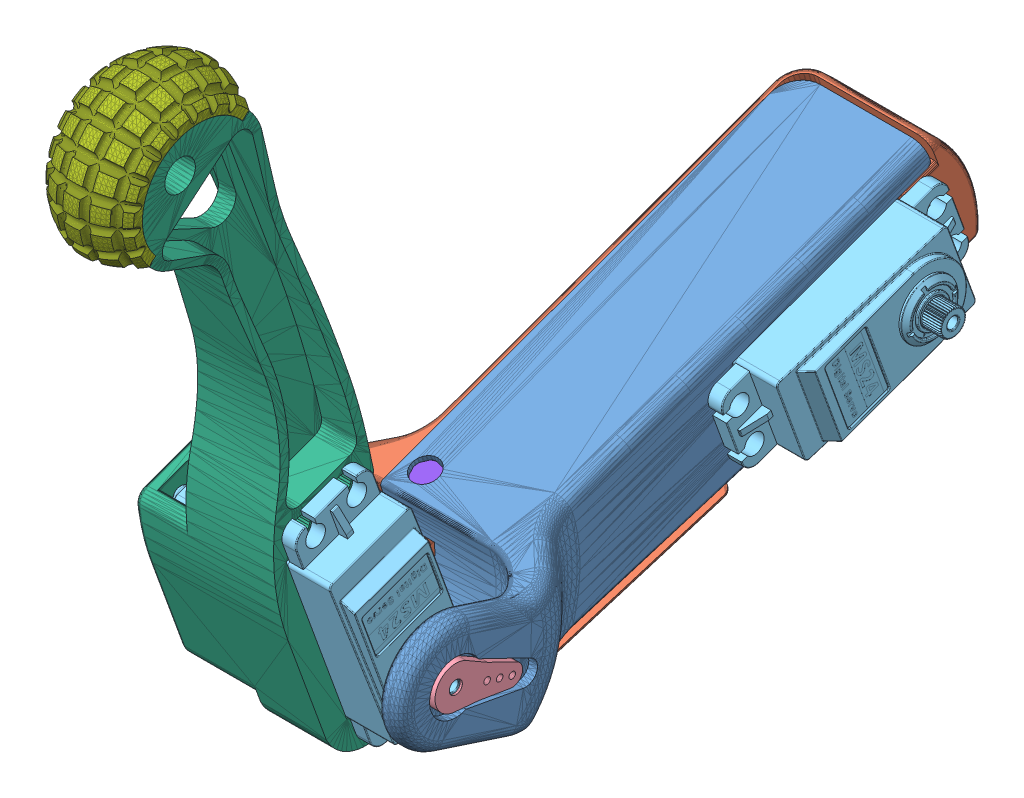
SolidWorks assembly Right Leg Assembly, configuration Default. Lengths in mm.
Overall size (64.22 167.45 199.81).
25 component instances, 9 part files, 59 mates.
Components (placement in the parent):
- Right_arm_joint_mg-1: Right_arm_joint_mg [Default] at (24.2858 18.5405 -25.0321) size (37.5 46 56.5) (hidden)
- Servohorn-1: Servohorn [4 Prong] at (-38.4142 28.7905 -4.7821) x (0 0.715501 0.698611) z (-1 0 0) size (31.8 31.8 2.24) (hidden)
- Servo Motor-1: Servo Motor [Default] at (-15.7142 38.5405 -14.5321) size (20.1 45.99 55.6) (hidden)
- Servohorn-2: Servohorn [Default] at (-15.7142 58.9405 -14.5321) x (-0.99999 0 0.00451) z (0 -1 0) size (28.18 31.8 2.24) (hidden)
- Right_arm_mg-1: Right_arm_mg [Default] at (-8.8142 41.6076 -10.7588) x (0 -0.939693 -0.34202) z (0 -0.34202 0.939693) size (38.24 39.8 137.4)
- SM_Right_arm_cover-1: SM_Right_arm_cover [Default] at (-48.6142 49.0427 -16.5661) x (0 -0.939693 -0.34202) z (0 -0.34202 0.939693) size (41.16 45 143.55)
- F625ZZ Ball Bearing-1: F625ZZ Ball Bearing [Default] at (-98.6142 -2.6723 100.0196) x (0 0.0383 -0.999266) z (1 0 0) size (18 18 5)
- Servohorn-3: Servohorn [1 Prong] at (-48.8142 5.2058 100.4211) x (0 -0.953491 0.301422) z (-1 0 0) size (9.55 20.65 2.24)
- Servo Motor-2: Servo Motor [Default] at (-67.7142 5.2058 100.4211) x (0 -0.34202 0.939693) z (0 0.939693 0.34202) size (20.1 45.99 55.6)
- Servo Motor-3: Servo Motor [Default] at (-58.8142 28.7905 -4.7821) x (0 -0.939693 -0.34202) z (0 -0.34202 0.939693) size (20.1 45.99 55.6)
- Right_wrist_mg-1: Right_wrist_mg [Default] at (-67.7142 -0.7709 87.604) x (0 0.939693 0.34202) z (0 -0.34202 0.939693) size (149.99 36.9 30)
- foot-1: foot [Default] at (-67.7142 114.2242 140.0873) x (0 -0.656061 0.754708) z (0 -0.754708 -0.656061) size (38.32 20 19.41)
- _Hex_Screws-1: _Hex_Screws [H M4x20] at (-20.7142 41.7405 19.4679) x (-0.837169 0 -0.546944) z (-0.546944 0 0.837169) size (7 22.8 8.08) (hidden)
- _Hex_Screws-2: _Hex_Screws [H M4x20] at (-10.7142 41.7405 -28.5321) x (-0.837169 0 -0.546944) z (-0.546944 0 0.837169) size (7 22.8 8.08) (hidden)
- _Hex_Screws-3: _Hex_Screws [H M4x20] at (-10.7142 41.7405 19.4679) x (-0.99108 0 -0.133267) z (-0.133267 0 0.99108) size (7 22.8 8.08) (hidden)
- _Hex_Screws-4: _Hex_Screws [H M4x20] at (-20.7142 41.7405 -28.5321) x (0.837169 0 0.546944) z (0.546944 0 -0.837169) size (7 22.8 8.08) (hidden)
- _Hex_Screws-5: _Hex_Screws [H M4x20] at (-55.6142 28.8803 -19.6479) x (0 0.085299 -0.996355) z (0 0.996355 0.085299) size (7 22.8 8.08) (hidden)
- _Hex_Screws-8: _Hex_Screws [H M4x20] at (-55.6142 12.4633 25.4573) x (0 -0.381849 0.924225) z (0 -0.924225 -0.381849) size (7 22.8 8.08) (hidden)
- _Hex_Screws-9: _Hex_Screws [H M4x20] at (-55.6142 21.8603 28.8775) x (0 -0.381849 0.924225) z (0 -0.924225 -0.381849) size (7 22.8 8.08) (hidden)
- _Hex_Screws-10: _Hex_Screws [H M4x20] at (-64.5142 -9.66 100.3313) x (0 -0.381849 0.924225) z (0 -0.924225 -0.381849) size (7 22.8 8.08) (hidden)
- _Hex_Screws-11: _Hex_Screws [H M4x20] at (-64.5142 38.8655 107.3514) x (0 -0.381849 0.924225) z (0 -0.924225 -0.381849) size (7 22.8 8.08) (hidden)
- _Hex_Screws-12: _Hex_Screws [H M4x20] at (-64.5142 -6.2398 90.9344) x (0 -0.381849 0.924225) z (0 -0.924225 -0.381849) size (7 22.8 8.08) (hidden)
- _Hex_Screws-14: _Hex_Screws [H M4x20] at (-64.5142 35.4453 116.7483) x (0 -0.381849 0.924225) z (0 -0.924225 -0.381849) size (7 22.8 8.08) (hidden)
- _Hex_Screws-15: _Hex_Screws [H M4x20] at (-55.6142 38.2772 -16.2277) x (0 0.381849 -0.924225) z (0 0.924225 0.381849) size (7 22.8 8.08) (hidden)
- _Hex_Screws-19: _Hex_Screws [H M3x16] at (-83.8911 13.8209 71.432) x (0.19625 0.335369 -0.921419) z (-0.980554 0.067122 -0.184415) size (5.5 18 6.35)
Mates (geometry in assembly coordinates):
- Coincident1: coincident anti-aligned: plane of Right_arm_joint_mg-1 through (-40.4142 18.5405 -25.0321) normal (1 0 0); plane of Servohorn-1 through (-40.4142 28.7905 -4.7821) normal (-1 0 0)
- Angle2: planar angle = 0.069813 rad anti-aligned: plane of Right_arm_joint_mg-1 through (24.2858 29.9404 -17.8834) normal (0 0.847204 0.531268); plane of Servohorn-1 through (-40.4142 21.752 -2.4794) normal (0 -0.808081 -0.589071)
- Coincident4: coincident: point of Right_arm_joint_mg-1; line of Servohorn-1 through (-38.4142 28.7905 -4.7821) axis (1 0 0)
- Coincident5: coincident anti-aligned: plane of Right_arm_joint_mg-1 through (-25.7142 18.5405 -25.0321) normal (1 0 0); plane of Servo Motor-1 through (-25.7142 49.5405 -23.5321) normal (-1 0 0)
- Coincident6: coincident anti-aligned: plane of Right_arm_joint_mg-1 through (24.2858 11.0405 -25.0321) normal (0 1 0); plane of Servo Motor-1 through (-15.7142 11.0405 -14.5321) normal (0 -1 0)
- Distance2: distance = 0 mm anti-aligned: plane of Servo Motor-1 through (-25.7142 18.5405 15.4679) normal (0 0 1); plane of Right_arm_joint_mg-1 through (24.2858 18.5405 15.4679) normal (0 0 -1)
- Concentric1: concentric anti-aligned: cylinder of Servo Motor-1 through (-15.7142 52.9405 -14.5321) axis (0 1 0) radius 1.25; line of Servohorn-2 through (-15.7142 58.9405 -14.5321) axis (0 -1 0)
- Coincident8: coincident anti-aligned: plane of Servo Motor-1 through (-15.7142 56.9405 -14.5321) normal (0 1 0); plane of Servohorn-2 through (-15.7142 56.9405 -14.5321) normal (0 -1 0)
- Coincident14: coincident anti-aligned: plane of Right_arm_mg-1 through (-88.6142 41.6076 -10.7588) normal (-1 0 0); plane of SM_Right_arm_cover-1 through (-88.6142 49.0427 -16.5661) normal (1 0 0)
- Distance4: distance = 1 mm aligned: plane of Right_arm_mg-1 through (-8.8142 41.6076 -10.7588) normal (0 -0.34202 0.939693); plane of SM_Right_arm_cover-1 through (-48.6142 46.6485 -9.9883) normal (0 -0.34202 0.939693)
- Coincident16: coincident aligned: plane of Right_arm_mg-1 through (-8.8142 20.9865 -18.2643) normal (0 -0.939693 -0.34202); plane of SM_Right_arm_cover-1 through (-48.6142 23.7227 -25.7819) normal (0 -0.939693 -0.34202)
- Tangent1: tangent anti-aligned: plane of SM_Right_arm_cover-1 through (-58.6142 8.2907 92.877) normal (0 -0.30578 0.952102); cylinder of F625ZZ Ball Bearing-1 through (-101.6142 5.3219 100.326) axis (-1 0 0) radius 8
- Coincident17: coincident anti-aligned: plane of SM_Right_arm_cover-1 through (-99.6142 49.0427 -16.5661) normal (1 0 0); plane of F625ZZ Ball Bearing-1 through (-99.6142 13.316 100.6324) normal (-1 0 0)
- Tangent4: tangent anti-aligned: plane of SM_Right_arm_cover-1 through (-58.6142 13.3121 99.5229) normal (0 -0.98251 0.186209); cylinder of F625ZZ Ball Bearing-1 through (-101.6142 5.3219 100.326) axis (-1 0 0) radius 8
- Coincident18: coincident anti-aligned: plane of Right_arm_mg-1 through (-50.8142 41.6076 -10.7588) normal (1 0 0); plane of Servohorn-3 through (-50.8142 5.2058 100.4211) normal (-1 0 0)
- Coincident19: coincident: point of Right_arm_mg-1; line of Servohorn-3 through (-48.8142 5.2058 100.4211) axis (-1 0 0)
- Parallel3: parallel anti-aligned: plane of Right_arm_mg-1 through (-8.8142 -26.9471 22.3339) normal (0 -0.900565 0.434721); plane of Servohorn-3 through (-50.8142 6.495 93.1286) normal (0 0.900565 -0.434721)
- Concentric2: concentric anti-aligned: line of Servohorn-1 through (-38.4142 28.7905 -4.7821) axis (-1 0 0); cylinder of Servo Motor-3 through (-44.4142 28.7905 -4.7821) axis (1 0 0) radius 1.25
- Coincident21: coincident anti-aligned: plane of Servohorn-1 through (-40.4142 28.7905 -4.7821) normal (-1 0 0); plane of Servo Motor-3 through (-40.4142 28.7905 -4.7821) normal (1 0 0)
- Coincident23: coincident anti-aligned: plane of Right_arm_mg-1 through (-8.8142 41.6076 -10.7588) normal (0 -0.939693 -0.34202); plane of Servo Motor-3 through (-47.8142 41.2656 -9.8191) normal (0 0.939693 0.34202)
- Coincident24: coincident anti-aligned: plane of Right_arm_mg-1 through (-8.8142 41.6076 -10.7588) normal (0 -0.34202 0.939693); plane of Servo Motor-3 through (-78.8142 41.6076 -10.7588) normal (0 0.34202 -0.939693)
- Coincident25: coincident anti-aligned: plane of Right_arm_mg-1 through (-58.8142 41.6076 -10.7588) normal (1 0 0); plane of Servo Motor-3 through (-58.8142 11.0987 17.5114) normal (-1 0 0)
- Coincident26: coincident anti-aligned: plane of Servo Motor-2 through (-67.7142 27.4993 118.1129) normal (-1 0 0); plane of Right_wrist_mg-1 through (-67.7142 -0.7709 87.604) normal (1 0 0)
- Coincident27: coincident anti-aligned: plane of Servo Motor-2 through (-87.7142 -0.7709 87.604) normal (0 -0.939693 -0.34202); plane of Right_wrist_mg-1 through (-67.7142 -0.7709 87.604) normal (0 0.939693 0.34202)
- Coincident29: coincident anti-aligned: plane of Servo Motor-2 through (-56.7142 29.0367 119.7367) normal (0 -0.34202 0.939693); plane of Right_wrist_mg-1 through (-67.7142 -7.6113 106.3979) normal (0 0.34202 -0.939693)
- Concentric3: concentric aligned: line of Servohorn-3 through (-48.8142 5.2058 100.4211) axis (1 0 0); cylinder of Servo Motor-2 through (-53.3142 5.2058 100.4211) axis (1 0 0) radius 1.25
- Distance6: distance = 1.5 mm anti-aligned: plane of Servohorn-3 through (-50.8142 5.2058 100.4211) normal (-1 0 0); plane of Servo Motor-2 through (-49.3142 5.2058 100.4211) normal (1 0 0)
- Coincident31: coincident anti-aligned: plane of Right_wrist_mg-1 through (-67.7142 50.7034 176.7608) normal (0 -0.499997 -0.866027); plane of foot-1 through (-67.7142 114.2242 140.0873) normal (0 0.499997 0.866027)
- Coincident32: coincident aligned: plane of Right_wrist_mg-1 through (-87.7142 -0.7709 87.604) normal (-1 0 0); plane of foot-1 through (-87.7142 114.2242 140.0873) normal (-1 0 0)
- Coincident34: coincident: point of Right_wrist_mg-1; line of foot-1 through (-87.7142 124.0354 148.6161) axis (0 0.629912 -0.776667)
- Concentric4: concentric aligned: cylinder of Servo Motor-1 through (-10.7142 32.1765 19.4679) axis (0 1 0) radius 2.25; cylinder of _Hex_Screws-3 through (-10.7142 21.7405 19.4679) axis (0 1 0) radius 2
- Coincident35: coincident anti-aligned: plane of Servo Motor-1 through (-15.7142 41.7405 -14.5321) normal (0 1 0); plane of _Hex_Screws-3 through (-10.7142 41.7405 19.4679) normal (0 -1 0)
- Concentric5: concentric aligned: cylinder of Servo Motor-1 through (-20.7142 32.1765 19.4679) axis (0 1 0) radius 2.25; cylinder of _Hex_Screws-1 through (-20.7142 21.7405 19.4679) axis (0 1 0) radius 2
- Coincident36: coincident aligned: plane of _Hex_Screws-1 through (-20.7142 44.5405 19.4679) normal (0 1 0); plane of _Hex_Screws-3 through (-10.7142 44.5405 19.4679) normal (0 1 0)
- Concentric6: concentric aligned: cylinder of Servo Motor-1 through (-20.7142 32.1765 -28.5321) axis (0 1 0) radius 2.25; cylinder of _Hex_Screws-4 through (-20.7142 21.7405 -28.5321) axis (0 1 0) radius 2
- Coincident37: coincident anti-aligned: plane of Servo Motor-1 through (-15.7142 41.7405 -14.5321) normal (0 1 0); plane of _Hex_Screws-4 through (-20.7142 41.7405 -28.5321) normal (0 -1 0)
- Concentric7: concentric aligned: cylinder of Servo Motor-1 through (-10.7142 32.1765 -28.5321) axis (0 1 0) radius 2.25; cylinder of _Hex_Screws-2 through (-10.7142 21.7405 -28.5321) axis (0 1 0) radius 2
- Coincident38: coincident anti-aligned: plane of Servo Motor-1 through (-15.7142 41.7405 -14.5321) normal (0 1 0); plane of _Hex_Screws-2 through (-10.7142 41.7405 -28.5321) normal (0 -1 0)
- Concentric8: concentric aligned: cylinder of Servo Motor-3 through (-65.1781 12.4633 25.4573) axis (1 0 0) radius 2.25; cylinder of _Hex_Screws-8 through (-75.6142 12.4633 25.4573) axis (1 0 0) radius 2
- Coincident39: coincident anti-aligned: plane of Servo Motor-3 through (-55.6142 28.7905 -4.7821) normal (1 0 0); plane of _Hex_Screws-8 through (-55.6142 12.4633 25.4573) normal (-1 0 0)
- Concentric9: concentric aligned: cylinder of Servo Motor-3 through (-65.1781 21.8603 28.8775) axis (1 0 0) radius 2.25; cylinder of _Hex_Screws-9 through (-75.6142 21.8603 28.8775) axis (1 0 0) radius 2
- Coincident40: coincident aligned: plane of _Hex_Screws-8 through (-52.8142 12.4633 25.4573) normal (1 0 0); plane of _Hex_Screws-9 through (-52.8142 21.8603 28.8775) normal (1 0 0)
- Concentric10: concentric aligned: cylinder of Servo Motor-3 through (-65.1781 28.8803 -19.6479) axis (1 0 0) radius 2.25; cylinder of _Hex_Screws-5 through (-75.6142 28.8803 -19.6479) axis (1 0 0) radius 2
- Coincident41: coincident anti-aligned: plane of Servo Motor-3 through (-55.6142 28.7905 -4.7821) normal (1 0 0); plane of _Hex_Screws-5 through (-55.6142 28.8803 -19.6479) normal (-1 0 0)
- Coincident42: coincident aligned: plane of _Hex_Screws-5 through (-52.8142 28.8803 -19.6479) normal (1 0 0); plane of _Hex_Screws-15 through (-52.8142 38.2772 -16.2277) normal (1 0 0)
- Concentric11: concentric aligned: cylinder of Servo Motor-3 through (-65.1781 38.2772 -16.2277) axis (1 0 0) radius 2.25; cylinder of _Hex_Screws-15 through (-75.6142 38.2772 -16.2277) axis (1 0 0) radius 2
- Concentric12: concentric aligned: cylinder of Servo Motor-2 through (-74.0781 38.8655 107.3514) axis (1 0 0) radius 2.25; cylinder of _Hex_Screws-11 through (-84.5142 38.8655 107.3514) axis (1 0 0) radius 2
- Concentric13: concentric aligned: cylinder of Servo Motor-2 through (-74.0781 35.4453 116.7483) axis (1 0 0) radius 2.25; cylinder of _Hex_Screws-14 through (-84.5142 35.4453 116.7483) axis (1 0 0) radius 2
- Concentric14: concentric aligned: cylinder of Servo Motor-2 through (-74.0781 -6.2398 90.9344) axis (1 0 0) radius 2.25; cylinder of _Hex_Screws-12 through (-84.5142 -6.2398 90.9344) axis (1 0 0) radius 2
- Concentric15: concentric aligned: cylinder of Servo Motor-2 through (-74.0781 -9.66 100.3313) axis (1 0 0) radius 2.25; cylinder of _Hex_Screws-10 through (-84.5142 -9.66 100.3313) axis (1 0 0) radius 2
- Coincident43: coincident aligned: plane of _Hex_Screws-10 through (-61.7142 -9.66 100.3313) normal (1 0 0); plane of _Hex_Screws-12 through (-61.7142 -6.2398 90.9344) normal (1 0 0)
- Coincident44: coincident aligned: plane of _Hex_Screws-10 through (-61.7142 -9.66 100.3313) normal (1 0 0); plane of _Hex_Screws-14 through (-61.7142 35.4453 116.7483) normal (1 0 0)
- Coincident45: coincident aligned: plane of _Hex_Screws-11 through (-61.7142 38.8655 107.3514) normal (1 0 0); plane of _Hex_Screws-14 through (-61.7142 35.4453 116.7483) normal (1 0 0)
- Coincident46: coincident anti-aligned: plane of Servo Motor-2 through (-64.5142 5.2058 100.4211) normal (1 0 0); plane of _Hex_Screws-11 through (-64.5142 38.8655 107.3514) normal (-1 0 0)
- Coincident47: coincident anti-aligned: plane of Right_arm_mg-1 through (-8.8142 43.487 -10.0748) normal (0 0.939693 0.34202); plane of _Hex_Screws-19 through (-83.8911 13.8209 71.432) normal (0 -0.939693 -0.34202)
- Tangent8: tangent anti-aligned: plane of Right_arm_mg-1 through (-95.3246 37.7119 -0.0555) normal (0.991443 0.044646 -0.122665); cylinder of _Hex_Screws-19 through (-83.8911 -1.2141 65.9597) axis (0 0.939693 0.34202) radius 1.5
- Tangent9: tangent anti-aligned: plane of Right_arm_mg-1 through (-21.5151 8.6152 79.8872) normal (0.130539 0.339094 -0.931652); cylinder of _Hex_Screws-19 through (-83.8911 -1.2141 65.9597) axis (0 0.939693 0.34202) radius 1.5
- Angle3: planar angle = 0.349066 rad aligned: plane of Right_arm_joint_mg-1 through (24.2858 18.5405 -33.0321) normal (0 0 -1); plane of Right_arm_mg-1 through (-8.8142 44.3438 -18.2764) normal (0 0.34202 -0.939693)
- Angle4: planar angle = 1.570796 rad anti-aligned: plane of Servo Motor-2 through (-56.7142 0.1688 87.946) normal (0 0.34202 -0.939693); plane of Right_arm_mg-1 through (-8.8142 46.3061 -9.0487) normal (0 0.939693 0.34202)
